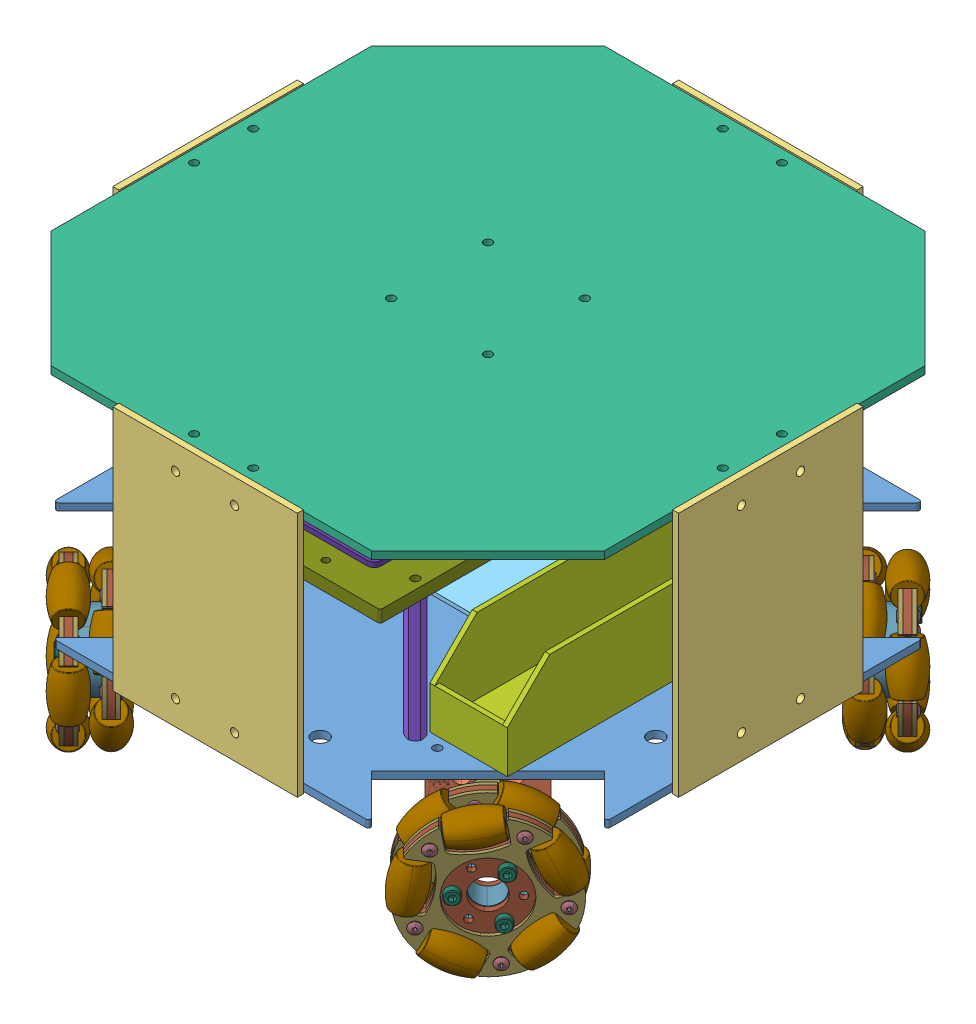
SolidWorks assembly ouijabot, configuration Default. Lengths in mm. (continued)
Components (placement in the parent): (continued)
- tx2-carrier-orbitty-1: tx2-carrier-orbitty [Default] at (43.5 74 -33.48) x (-1 0 0) z (0 -1 0) size (87.04 52.68 23.65) (continued)
  - ASG003_3D_MODEL.step-1: ASG003_3D_MODEL.step [Default] at origin size (87.04 52.68 23.65) (continued)
    - U8.step-1: U8.step [Default] at origin size (1.26 2.01 0.91) (continued)
      - 870945920.step-1: 870945920.step [Default] at (17.6522 30.9566 -2.6006) size (1.26 2.01 0.91) (continued)
        - Extruded-6.step-1: Extruded-6.step [Default] at origin size (1.26 2.01 0.91)
    - U4.step-1: U4.step [Default] at origin size (3 1.7 1.45)
      - 870946240.step-1: 870946240.step [Default] at (13.3342 34.2586 -3.0506) size (3 1.7 1.45)
        - Extruded-8.step-1: Extruded-8.step [Default] at origin size (3 1.7 1.45)
    - S1.step-1: S1.step [Default] at origin size (8.13 3.66 2.38)
      - 870942400.step-1: 870942400.step [Default] at (63.7532 2.3346 1.27) size (3.81 1.02 1.07)
        - Extruded-9.step-1: Extruded-9.step [Default] at origin size (3.81 1.02 1.07)
      - 870942560.step-1: 870942560.step [Default] at (63.7532 2.3346 1.27) size (2.54 0.76 1.09)
        - Extruded-10.step-1: Extruded-10.step [Default] at origin size (2.54 0.76 1.09)
      - 870942720.step-1: 870942720.step [Default] at (64.3247 2.3346 1.27) size (1.14 0.51 1.12)
        - Extruded-11.step-1: Extruded-11.step [Default] at origin size (1.14 0.51 1.12)
      - 870942720.step-2: 870942720.step [Default] at (63.1817 3.6046 1.27) size (1.14 0.51 1.12)
        - Extruded-11.step-1: Extruded-11.step [Default] at origin size (1.14 0.51 1.12)
      - 870942560.step-2: 870942560.step [Default] at (63.7532 3.6046 1.27) size (2.54 0.76 1.09)
        - Extruded-10.step-1: Extruded-10.step [Default] at origin size (2.54 0.76 1.09)
      - 870942400.step-2: 870942400.step [Default] at (63.7532 3.6046 1.27) size (3.81 1.02 1.07)
        - Extruded-9.step-1: Extruded-9.step [Default] at origin size (3.81 1.02 1.07)
      - c-1571983-01-b-3d.step-1: c-1571983-01-b-3d.step [Default] at (63.7533 2.9696 0.571) x (0 1 0) z (0 0 1) size (3.66 8.13 2.31)
    - R50.step-1: R50.step [Default] at origin size (0.52 1.02 0.36)
      - 870941120.step-1: 870941120.step [Default] at (22.2242 30.5266 -1.9516) size (0.52 0.16 0.35)
        - Extruded-1.step-1: Extruded-1.step [Default] at origin size (0.52 0.16 0.35)
      - 870941120.step-2: 870941120.step [Default] at (22.2242 31.3866 -1.9516) size (0.52 0.16 0.35)
        - Extruded-1.step-1: Extruded-1.step [Default] at origin size (0.52 0.16 0.35)
      - 870941280.step-1: 870941280.step [Default] at (22.2242 30.9566 -1.9506) size (0.51 1.01 0.36)
        - Extruded-2.step-1: Extruded-2.step [Default] at origin size (0.51 1.01 0.36)
    - R49.step-1: R49.step [Default] at origin size (0.52 1.02 0.36)
      - 870941120.step-1: 870941120.step [Default] at (20.9542 37.8636 -1.9516) size (0.52 0.16 0.35)
        - Extruded-1.step-1: Extruded-1.step [Default] at origin size (0.52 0.16 0.35)
      - 870941120.step-2: 870941120.step [Default] at (20.9542 37.0036 -1.9516) size (0.52 0.16 0.35)
        - Extruded-1.step-1: Extruded-1.step [Default] at origin size (0.52 0.16 0.35)
      - 870941280.step-1: 870941280.step [Default] at (20.9542 37.4336 -1.9506) size (0.51 1.01 0.36)
        - Extruded-2.step-1: Extruded-2.step [Default] at origin size (0.51 1.01 0.36)
    - R48.step-1: R48.step [Default] at origin size (0.52 1.02 0.36)
      - 870941120.step-1: 870941120.step [Default] at (21.0812 31.3866 -1.9516) size (0.52 0.16 0.35)
        - Extruded-1.step-1: Extruded-1.step [Default] at origin size (0.52 0.16 0.35)
      - 870941120.step-2: 870941120.step [Default] at (21.0812 30.5266 -1.9516) size (0.52 0.16 0.35)
        - Extruded-1.step-1: Extruded-1.step [Default] at origin size (0.52 0.16 0.35)
      - 870941280.step-1: 870941280.step [Default] at (21.0812 30.9566 -1.9506) size (0.51 1.01 0.36)
        - Extruded-2.step-1: Extruded-2.step [Default] at origin size (0.51 1.01 0.36)
    - R22.step-1: R22.step [Default] at origin size (0.52 1.02 0.36)
      - 870941120.step-1: 870941120.step [Default] at (15.3662 32.0216 -1.9516) size (0.52 0.16 0.35)
        - Extruded-1.step-1: Extruded-1.step [Default] at origin size (0.52 0.16 0.35)
      - 870941120.step-2: 870941120.step [Default] at (15.3662 31.1616 -1.9516) size (0.52 0.16 0.35)
        - Extruded-1.step-1: Extruded-1.step [Default] at origin size (0.52 0.16 0.35)
      - 870941280.step-1: 870941280.step [Default] at (15.3662 31.5916 -1.9506) size (0.51 1.01 0.36)
        - Extruded-2.step-1: Extruded-2.step [Default] at origin size (0.51 1.01 0.36)
    - R18.step-1: R18.step [Default] at origin size (0.52 1.02 0.36)
      - 870941120.step-1: 870941120.step [Default] at (78.867 21.795 -1.9516) size (0.52 0.16 0.35)
        - Extruded-1.step-1: Extruded-1.step [Default] at origin size (0.52 0.16 0.35)
      - 870941120.step-2: 870941120.step [Default] at (78.867 22.655 -1.9516) size (0.52 0.16 0.35)
        - Extruded-1.step-1: Extruded-1.step [Default] at origin size (0.52 0.16 0.35)
      - 870941280.step-1: 870941280.step [Default] at (78.867 22.225 -1.9506) size (0.51 1.01 0.36)
        - Extruded-2.step-1: Extruded-2.step [Default] at origin size (0.51 1.01 0.36)
    - L7.step-1: L7.step [Default] at origin size (1.6 0.9 0.46)
      - 870942240.step-1: 870942240.step [Default] at (75.692 25.273 -2.0506) size (1 0.9 0.45)
        - Extruded-12.step-1: Extruded-12.step [Default] at origin size (1 0.9 0.45)
      - 870942080.step-1: 870942080.step [Default] at (76.342 25.273 -2.0606) size (0.3 0.9 0.46)
        - Extruded-13.step-1: Extruded-13.step [Default] at origin size (0.3 0.9 0.46)
      - 870942080.step-2: 870942080.step [Default] at (75.042 25.273 -2.0606) size (0.3 0.9 0.46)
        - Extruded-13.step-1: Extruded-13.step [Default] at origin size (0.3 0.9 0.46)
    - C58.step-1: C58.step [Default] at origin size (0.52 1.02 0.36)
      - 870941120.step-1: 870941120.step [Default] at (19.9382 31.3866 -1.9516) size (0.52 0.16 0.35)
        - Extruded-1.step-1: Extruded-1.step [Default] at origin size (0.52 0.16 0.35)
      - 870941120.step-2: 870941120.step [Default] at (19.9382 30.5266 -1.9516) size (0.52 0.16 0.35)
        - Extruded-1.step-1: Extruded-1.step [Default] at origin size (0.52 0.16 0.35)
      - 870941280.step-1: 870941280.step [Default] at (19.9382 30.9566 -1.9506) size (0.51 1.01 0.36)
        - Extruded-2.step-1: Extruded-2.step [Default] at origin size (0.51 1.01 0.36)
    - C50.step-1: C50.step [Default] at origin size (0.52 1.02 0.36)
      - 870941120.step-1: 870941120.step [Default] at (12.4452 36.7496 -1.9516) size (0.52 0.16 0.35)
        - Extruded-1.step-1: Extruded-1.step [Default] at origin size (0.52 0.16 0.35)
      - 870941120.step-2: 870941120.step [Default] at (12.4452 37.6096 -1.9516) size (0.52 0.16 0.35)
        - Extruded-1.step-1: Extruded-1.step [Default] at origin size (0.52 0.16 0.35)
      - 870941280.step-1: 870941280.step [Default] at (12.4452 37.1796 -1.9506) size (0.51 1.01 0.36)
        - Extruded-2.step-1: Extruded-2.step [Default] at origin size (0.51 1.01 0.36)
    - C49.step-1: C49.step [Default] at origin size (0.52 1.02 0.36)
      - 870941120.step-1: 870941120.step [Default] at (14.3502 36.8076 -1.9516) size (0.52 0.16 0.35)
        - Extruded-1.step-1: Extruded-1.step [Default] at origin size (0.52 0.16 0.35)
      - 870941120.step-2: 870941120.step [Default] at (14.3502 37.6676 -1.9516) size (0.52 0.16 0.35)
        - Extruded-1.step-1: Extruded-1.step [Default] at origin size (0.52 0.16 0.35)
      - 870941280.step-1: 870941280.step [Default] at (14.3502 37.2376 -1.9506) size (0.51 1.01 0.36)
        - Extruded-2.step-1: Extruded-2.step [Default] at origin size (0.51 1.01 0.36)
    - C48.step-1: C48.step [Default] at origin size (1.02 0.52 0.36)
      - 870940480.step-1: 870940480.step [Default] at (84.533 22.733 0) size (0.16 0.52 0.35)
        - Extruded.step-1: Extruded.step [Default] at origin size (0.16 0.52 0.35)
      - 870940480.step-2: 870940480.step [Default] at (85.393 22.733 0) size (0.16 0.52 0.35)
        - Extruded.step-1: Extruded.step [Default] at origin size (0.16 0.52 0.35)
      - 870940640.step-1: 870940640.step [Default] at (84.963 22.733 0) size (1.01 0.51 0.36)
        - Extruded-0.step-1: Extruded-0.step [Default] at origin size (1.01 0.51 0.36)
    - R47.step-1: R47.step [Default] at origin size (1.02 0.52 0.36)
      - 870940480.step-1: 870940480.step [Default] at (63.9292 23.9246 0) size (0.16 0.52 0.35)
        - Extruded.step-1: Extruded.step [Default] at origin size (0.16 0.52 0.35)
      - 870940480.step-2: 870940480.step [Default] at (63.0692 23.9246 0) size (0.16 0.52 0.35)
        - Extruded.step-1: Extruded.step [Default] at origin size (0.16 0.52 0.35)
      - 870940640.step-1: 870940640.step [Default] at (63.4992 23.9246 0) size (1.01 0.51 0.36)
        - Extruded-0.step-1: Extruded-0.step [Default] at origin size (1.01 0.51 0.36)
    - R46.step-1: R46.step [Default] at origin size (0.52 1.02 0.36)
      - 870941120.step-1: 870941120.step [Default] at (8.255 20.017 0) size (0.52 0.16 0.35)
        - Extruded-1.step-1: Extruded-1.step [Default] at origin size (0.52 0.16 0.35)
      - 870941120.step-2: 870941120.step [Default] at (8.255 20.877 0) size (0.52 0.16 0.35)
        - Extruded-1.step-1: Extruded-1.step [Default] at origin size (0.52 0.16 0.35)
      - 870941280.step-1: 870941280.step [Default] at (8.255 20.447 0) size (0.51 1.01 0.36)
        - Extruded-2.step-1: Extruded-2.step [Default] at origin size (0.51 1.01 0.36)
    - L1.step-1: L1.step [Default] at origin size (1 1.25 0.29)
      - 870940800.step-1: 870940800.step [Default] at (44.881 29.538 0.005) size (1 1.25 0.29)
        - Extruded-14.step-1: Extruded-14.step [Default] at origin size (1 1.25 0.29)
    - U7.step-1: U7.step [Default] at origin size (1.6 3 1.1)
      - 870944800.step-1: 870944800.step [Default] at (65.913 27.94 0) size (1.6 3 1.1)
        - Extruded-15.step-1: Extruded-15.step [Default] at origin size (1.6 3 1.1)
    - U5.step-1: U5.step [Default] at origin size (3.1 3.1 0.95)
      - 870940320.step-1: 870940320.step [Default] at (30.2506 29.8936 0.05) size (3.1 3.1 0.95)
        - Extruded-16.step-1: Extruded-16.step [Default] at origin size (3.1 3.1 0.95)
    - U3.step-1: U3.step [Default] at origin size (3.65 3.65 0.95)
      - 870946080.step-1: 870946080.step [Default] at (8.751 30.152 -2.6006) size (3.65 3.65 0.95)
        - Extruded-17.step-1: Extruded-17.step [Default] at origin size (3.65 3.65 0.95)
    - U2.step-1: U2.step [Default] at origin size (3.65 3.65 0.95)
      - 870946080.step-1: 870946080.step [Default] at (8.751 37.539 -2.6006) size (3.65 3.65 0.95)
        - Extruded-17.step-1: Extruded-17.step [Default] at origin size (3.65 3.65 0.95)
    - U1.step-1: U1.step [Default] at origin size (4.1 4.1 0.5)
      - 870941920.step-1: 870941920.step [Default] at (55.7522 32.8146 0) size (4.1 4.1 0.5)
        - Extruded-18.step-1: Extruded-18.step [Default] at origin size (4.1 4.1 0.5)
    - SW3.step-1: SW3.step [Default] at origin size (4.6 2.8 1.9)
      - 870942880.step-1: 870942880.step [Default] at (44.9573 2.8427 0) size (4.6 2.8 1.4)
        - Extruded-19.step-1: Extruded-19.step [Default] at origin size (4.6 2.8 1.4)
      - 870943040.step-1: 870943040.step [Default] at (44.9572 2.8426 1.4) size (2.2 1.6 0.5)
        - Extruded-20.step-1: Extruded-20.step [Default] at origin size (2.2 1.6 0.5)
    - SW2.step-1: SW2.step [Default] at origin size (4.6 2.8 1.9)
      - 870942880.step-1: 870942880.step [Default] at (53.0853 2.8427 0) size (4.6 2.8 1.4)
        - Extruded-19.step-1: Extruded-19.step [Default] at origin size (4.6 2.8 1.4)
      - 870943040.step-1: 870943040.step [Default] at (53.0852 2.8426 1.4) size (2.2 1.6 0.5)
        - Extruded-20.step-1: Extruded-20.step [Default] at origin size (2.2 1.6 0.5)
    - SW1.step-1: SW1.step [Default] at origin size (4.6 2.8 1.9)
      - 870942880.step-1: 870942880.step [Default] at (36.8293 2.8427 0) size (4.6 2.8 1.4)
        - Extruded-19.step-1: Extruded-19.step [Default] at origin size (4.6 2.8 1.4)
      - 870943040.step-1: 870943040.step [Default] at (36.8292 2.8426 1.4) size (2.2 1.6 0.5)
        - Extruded-20.step-1: Extruded-20.step [Default] at origin size (2.2 1.6 0.5)
    - R45.step-1: R45.step [Default] at origin size (1.02 0.52 0.36)
      - 870940480.step-1: 870940480.step [Default] at (64.6964 25.5915 0) size (0.16 0.52 0.35)
        - Extruded.step-1: Extruded.step [Default] at origin size (0.16 0.52 0.35)
      - 870940480.step-2: 870940480.step [Default] at (65.5564 25.5915 0) size (0.16 0.52 0.35)
        - Extruded.step-1: Extruded.step [Default] at origin size (0.16 0.52 0.35)
      - 870940640.step-1: 870940640.step [Default] at (65.1264 25.5915 0) size (1.01 0.51 0.36)
        - Extruded-0.step-1: Extruded-0.step [Default] at origin size (1.01 0.51 0.36)
    - R44.step-1: R44.step [Default] at origin size (1.02 0.52 0.36)
      - 870940480.step-1: 870940480.step [Default] at (66.4744 25.5915 0) size (0.16 0.52 0.35)
        - Extruded.step-1: Extruded.step [Default] at origin size (0.16 0.52 0.35)
      - 870940480.step-2: 870940480.step [Default] at (67.3344 25.5915 0) size (0.16 0.52 0.35)
        - Extruded.step-1: Extruded.step [Default] at origin size (0.16 0.52 0.35)
      - 870940640.step-1: 870940640.step [Default] at (66.9044 25.5915 0) size (1.01 0.51 0.36)
        - Extruded-0.step-1: Extruded-0.step [Default] at origin size (1.01 0.51 0.36)
    - R39.step-1: R39.step [Default] at origin size (1.6 0.9 0.46)
      - 870942080.step-1: 870942080.step [Default] at (83.581 19.304 0) size (0.3 0.9 0.46)
        - Extruded-13.step-1: Extruded-13.step [Default] at origin size (0.3 0.9 0.46)
      - 870942080.step-2: 870942080.step [Default] at (82.281 19.304 0) size (0.3 0.9 0.46)
        - Extruded-13.step-1: Extruded-13.step [Default] at origin size (0.3 0.9 0.46)
      - 870942240.step-1: 870942240.step [Default] at (82.931 19.304 0) size (1 0.9 0.45)
        - Extruded-12.step-1: Extruded-12.step [Default] at origin size (1 0.9 0.45)
    - R38.step-1: R38.step [Default] at origin size (1.02 0.52 0.36)
      - 870940480.step-1: 870940480.step [Default] at (67.3872 19.3526 -1.9516) size (0.16 0.52 0.35)
        - Extruded.step-1: Extruded.step [Default] at origin size (0.16 0.52 0.35)
      - 870940480.step-2: 870940480.step [Default] at (68.2472 19.3526 -1.9516) size (0.16 0.52 0.35)
        - Extruded.step-1: Extruded.step [Default] at origin size (0.16 0.52 0.35)
      - 870940640.step-1: 870940640.step [Default] at (67.8172 19.3526 -1.9506) size (1.01 0.51 0.36)
        - Extruded-0.step-1: Extruded-0.step [Default] at origin size (1.01 0.51 0.36)
    - R37.step-1: R37.step [Default] at origin size (1.02 0.52 0.36)
      - 870940480.step-1: 870940480.step [Default] at (61.3892 19.3526 -1.9516) size (0.16 0.52 0.35)
        - Extruded.step-1: Extruded.step [Default] at origin size (0.16 0.52 0.35)
      - 870940480.step-2: 870940480.step [Default] at (60.5292 19.3526 -1.9516) size (0.16 0.52 0.35)
        - Extruded.step-1: Extruded.step [Default] at origin size (0.16 0.52 0.35)
      - 870940640.step-1: 870940640.step [Default] at (60.9592 19.3526 -1.9506) size (1.01 0.51 0.36)
        - Extruded-0.step-1: Extruded-0.step [Default] at origin size (1.01 0.51 0.36)
    - R36.step-1: R36.step [Default] at origin size (1.02 0.52 0.36)
      - 870940480.step-1: 870940480.step [Default] at (64.9742 23.9246 0) size (0.16 0.52 0.35)
        - Extruded.step-1: Extruded.step [Default] at origin size (0.16 0.52 0.35)
      - 870940480.step-2: 870940480.step [Default] at (65.8342 23.9246 0) size (0.16 0.52 0.35)
        - Extruded.step-1: Extruded.step [Default] at origin size (0.16 0.52 0.35)
      - 870940640.step-1: 870940640.step [Default] at (65.4042 23.9246 0) size (1.01 0.51 0.36)
        - Extruded-0.step-1: Extruded-0.step [Default] at origin size (1.01 0.51 0.36)
    - R35.step-1: R35.step [Default] at origin size (0.52 1.02 0.36)
      - 870941120.step-1: 870941120.step [Default] at (32.0286 29.6596 -1.9516) size (0.52 0.16 0.35)
        - Extruded-1.step-1: Extruded-1.step [Default] at origin size (0.52 0.16 0.35)
      - 870941120.step-2: 870941120.step [Default] at (32.0286 30.5196 -1.9516) size (0.52 0.16 0.35)
        - Extruded-1.step-1: Extruded-1.step [Default] at origin size (0.52 0.16 0.35)
      - 870941280.step-1: 870941280.step [Default] at (32.0286 30.0896 -1.9506) size (0.51 1.01 0.36)
        - Extruded-2.step-1: Extruded-2.step [Default] at origin size (0.51 1.01 0.36)
    - R34.step-1: R34.step [Default] at origin size (1.02 0.52 0.36)
      - 870940480.step-1: 870940480.step [Default] at (32.865 28.6744 -1.9516) size (0.16 0.52 0.35)
        - Extruded.step-1: Extruded.step [Default] at origin size (0.16 0.52 0.35)
      - 870940480.step-2: 870940480.step [Default] at (32.005 28.6744 -1.9516) size (0.16 0.52 0.35)
        - Extruded.step-1: Extruded.step [Default] at origin size (0.16 0.52 0.35)
      - 870940640.step-1: 870940640.step [Default] at (32.435 28.6744 -1.9506) size (1.01 0.51 0.36)
        - Extruded-0.step-1: Extruded-0.step [Default] at origin size (1.01 0.51 0.36)
    - R33.step-1: R33.step [Default] at origin size (1.02 0.52 0.36)
      - 870940480.step-1: 870940480.step [Default] at (69.695 43.127 0) size (0.16 0.52 0.35)
        - Extruded.step-1: Extruded.step [Default] at origin size (0.16 0.52 0.35)
      - 870940480.step-2: 870940480.step [Default] at (68.835 43.127 0) size (0.16 0.52 0.35)
        - Extruded.step-1: Extruded.step [Default] at origin size (0.16 0.52 0.35)
      - 870940640.step-1: 870940640.step [Default] at (69.265 43.127 0) size (1.01 0.51 0.36)
        - Extruded-0.step-1: Extruded-0.step [Default] at origin size (1.01 0.51 0.36)
    - R32.step-1: R32.step [Default] at origin size (1.02 0.52 0.36)
      - 870940480.step-1: 870940480.step [Default] at (30.6806 31.2906 -1.9516) size (0.16 0.52 0.35)
        - Extruded.step-1: Extruded.step [Default] at origin size (0.16 0.52 0.35)
      - 870940480.step-2: 870940480.step [Default] at (29.8206 31.2906 -1.9516) size (0.16 0.52 0.35)
        - Extruded.step-1: Extruded.step [Default] at origin size (0.16 0.52 0.35)
      - 870940640.step-1: 870940640.step [Default] at (30.2506 31.2906 -1.9506) size (1.01 0.51 0.36)
        - Extruded-0.step-1: Extruded-0.step [Default] at origin size (1.01 0.51 0.36)
    - R31.step-1: R31.step [Default] at origin size (0.52 1.02 0.36)
      - 870941120.step-1: 870941120.step [Default] at (28.4726 29.7176 -1.9516) size (0.52 0.16 0.35)
        - Extruded-1.step-1: Extruded-1.step [Default] at origin size (0.52 0.16 0.35)
      - 870941120.step-2: 870941120.step [Default] at (28.4726 30.5776 -1.9516) size (0.52 0.16 0.35)
        - Extruded-1.step-1: Extruded-1.step [Default] at origin size (0.52 0.16 0.35)
      - 870941280.step-1: 870941280.step [Default] at (28.4726 30.1476 -1.9506) size (0.51 1.01 0.36)
        - Extruded-2.step-1: Extruded-2.step [Default] at origin size (0.51 1.01 0.36)
    - R30.step-1: R30.step [Default] at origin size (1.02 0.52 0.36)
      - 870940480.step-1: 870940480.step [Default] at (27.6362 28.6998 -1.9516) size (0.16 0.52 0.35)
        - Extruded.step-1: Extruded.step [Default] at origin size (0.16 0.52 0.35)
      - 870940480.step-2: 870940480.step [Default] at (28.4962 28.6998 -1.9516) size (0.16 0.52 0.35)
        - Extruded.step-1: Extruded.step [Default] at origin size (0.16 0.52 0.35)
      - 870940640.step-1: 870940640.step [Default] at (28.0662 28.6998 -1.9506) size (1.01 0.51 0.36)
        - Extruded-0.step-1: Extruded-0.step [Default] at origin size (1.01 0.51 0.36)
    - R29.step-1: R29.step [Default] at origin size (0.52 1.02 0.36)
      - 870941120.step-1: 870941120.step [Default] at (68.884 46.224 0) size (0.52 0.16 0.35)
        - Extruded-1.step-1: Extruded-1.step [Default] at origin size (0.52 0.16 0.35)
      - 870941120.step-2: 870941120.step [Default] at (68.884 45.364 0) size (0.52 0.16 0.35)
        - Extruded-1.step-1: Extruded-1.step [Default] at origin size (0.52 0.16 0.35)
      - 870941280.step-1: 870941280.step [Default] at (68.884 45.794 0) size (0.51 1.01 0.36)
        - Extruded-2.step-1: Extruded-2.step [Default] at origin size (0.51 1.01 0.36)
    - R28.step-1: R28.step [Default] at origin size (0.52 1.02 0.36)
      - 870941120.step-1: 870941120.step [Default] at (51.054 8.333 0) size (0.52 0.16 0.35)
        - Extruded-1.step-1: Extruded-1.step [Default] at origin size (0.52 0.16 0.35)
      - 870941120.step-2: 870941120.step [Default] at (51.054 9.193 0) size (0.52 0.16 0.35)
        - Extruded-1.step-1: Extruded-1.step [Default] at origin size (0.52 0.16 0.35)
      - 870941280.step-1: 870941280.step [Default] at (51.054 8.763 0) size (0.51 1.01 0.36)
        - Extruded-2.step-1: Extruded-2.step [Default] at origin size (0.51 1.01 0.36)
    - R27.step-1: R27.step [Default] at origin size (0.52 1.02 0.36)
      - 870941120.step-1: 870941120.step [Default] at (50.038 9.193 0) size (0.52 0.16 0.35)
        - Extruded-1.step-1: Extruded-1.step [Default] at origin size (0.52 0.16 0.35)
      - 870941120.step-2: 870941120.step [Default] at (50.038 8.333 0) size (0.52 0.16 0.35)
        - Extruded-1.step-1: Extruded-1.step [Default] at origin size (0.52 0.16 0.35)
      - 870941280.step-1: 870941280.step [Default] at (50.038 8.763 0) size (0.51 1.01 0.36)
        - Extruded-2.step-1: Extruded-2.step [Default] at origin size (0.51 1.01 0.36)
    - R26.step-1: R26.step [Default] at origin size (0.52 1.02 0.36)
      - 870941120.step-1: 870941120.step [Default] at (73.66 34.466 -1.9516) size (0.52 0.16 0.35)
        - Extruded-1.step-1: Extruded-1.step [Default] at origin size (0.52 0.16 0.35)
      - 870941120.step-2: 870941120.step [Default] at (73.66 33.606 -1.9516) size (0.52 0.16 0.35)
        - Extruded-1.step-1: Extruded-1.step [Default] at origin size (0.52 0.16 0.35)
      - 870941280.step-1: 870941280.step [Default] at (73.66 34.036 -1.9506) size (0.51 1.01 0.36)
        - Extruded-2.step-1: Extruded-2.step [Default] at origin size (0.51 1.01 0.36)
    - R25.step-1: R25.step [Default] at origin size (1.02 0.52 0.36)
      - 870940480.step-1: 870940480.step [Default] at (78.183 29.337 -1.9516) size (0.16 0.52 0.35)
        - Extruded.step-1: Extruded.step [Default] at origin size (0.16 0.52 0.35)
      - 870940480.step-2: 870940480.step [Default] at (79.043 29.337 -1.9516) size (0.16 0.52 0.35)
        - Extruded.step-1: Extruded.step [Default] at origin size (0.16 0.52 0.35)
      - 870940640.step-1: 870940640.step [Default] at (78.613 29.337 -1.9506) size (1.01 0.51 0.36)
        - Extruded-0.step-1: Extruded-0.step [Default] at origin size (1.01 0.51 0.36)
    - R24.step-1: R24.step [Default] at origin size (0.52 1.02 0.36)
      - 870941120.step-1: 870941120.step [Default] at (20.878 18.694 -1.9516) size (0.52 0.16 0.35)
        - Extruded-1.step-1: Extruded-1.step [Default] at origin size (0.52 0.16 0.35)
      - 870941120.step-2: 870941120.step [Default] at (20.878 19.554 -1.9516) size (0.52 0.16 0.35)
        - Extruded-1.step-1: Extruded-1.step [Default] at origin size (0.52 0.16 0.35)
      - 870941280.step-1: 870941280.step [Default] at (20.878 19.124 -1.9506) size (0.51 1.01 0.36)
        - Extruded-2.step-1: Extruded-2.step [Default] at origin size (0.51 1.01 0.36)
    - R23.step-1: R23.step [Default] at origin size (0.52 1.02 0.36)
      - 870941120.step-1: 870941120.step [Default] at (10.464 18.694 -1.9516) size (0.52 0.16 0.35)
        - Extruded-1.step-1: Extruded-1.step [Default] at origin size (0.52 0.16 0.35)
      - 870941120.step-2: 870941120.step [Default] at (10.464 19.554 -1.9516) size (0.52 0.16 0.35)
        - Extruded-1.step-1: Extruded-1.step [Default] at origin size (0.52 0.16 0.35)
      - 870941280.step-1: 870941280.step [Default] at (10.464 19.124 -1.9506) size (0.51 1.01 0.36)
        - Extruded-2.step-1: Extruded-2.step [Default] at origin size (0.51 1.01 0.36)
    - R20.step-1: R20.step [Default] at origin size (1.02 0.52 0.36)
      - 870940480.step-1: 870940480.step [Default] at (7.854 26.67 -1.9516) size (0.16 0.52 0.35)
        - Extruded.step-1: Extruded.step [Default] at origin size (0.16 0.52 0.35)
      - 870940480.step-2: 870940480.step [Default] at (6.994 26.67 -1.9516) size (0.16 0.52 0.35)
        - Extruded.step-1: Extruded.step [Default] at origin size (0.16 0.52 0.35)
      - 870940640.step-1: 870940640.step [Default] at (7.424 26.67 -1.9506) size (1.01 0.51 0.36)
        - Extruded-0.step-1: Extruded-0.step [Default] at origin size (1.01 0.51 0.36)
    - R21.step-1: R21.step [Default] at origin size (1.02 0.52 0.36)
      - 870940480.step-1: 870940480.step [Default] at (18.8442 37.0526 -1.9516) size (0.16 0.52 0.35)
        - Extruded.step-1: Extruded.step [Default] at origin size (0.16 0.52 0.35)
      - 870940480.step-2: 870940480.step [Default] at (17.9842 37.0526 -1.9516) size (0.16 0.52 0.35)
        - Extruded.step-1: Extruded.step [Default] at origin size (0.16 0.52 0.35)
      - 870940640.step-1: 870940640.step [Default] at (18.4142 37.0526 -1.9506) size (1.01 0.51 0.36)
        - Extruded-0.step-1: Extruded-0.step [Default] at origin size (1.01 0.51 0.36)
    - R19.step-1: R19.step [Default] at origin size (0.52 1.02 0.36)
      - 870941120.step-1: 870941120.step [Default] at (55.372 8.431 0) size (0.52 0.16 0.35)
        - Extruded-1.step-1: Extruded-1.step [Default] at origin size (0.52 0.16 0.35)
      - 870941120.step-2: 870941120.step [Default] at (55.372 7.571 0) size (0.52 0.16 0.35)
        - Extruded-1.step-1: Extruded-1.step [Default] at origin size (0.52 0.16 0.35)
      - 870941280.step-1: 870941280.step [Default] at (55.372 8.001 0) size (0.51 1.01 0.36)
        - Extruded-2.step-1: Extruded-2.step [Default] at origin size (0.51 1.01 0.36)
    - R15.step-1: R15.step [Default] at origin size (1.02 0.52 0.36)
      - 870940480.step-1: 870940480.step [Default] at (7.923 34.671 -1.9516) size (0.16 0.52 0.35)
        - Extruded.step-1: Extruded.step [Default] at origin size (0.16 0.52 0.35)
      - 870940480.step-2: 870940480.step [Default] at (7.063 34.671 -1.9516) size (0.16 0.52 0.35)
        - Extruded.step-1: Extruded.step [Default] at origin size (0.16 0.52 0.35)
      - 870940640.step-1: 870940640.step [Default] at (7.493 34.671 -1.9506) size (1.01 0.51 0.36)
        - Extruded-0.step-1: Extruded-0.step [Default] at origin size (1.01 0.51 0.36)
    - R17.step-1: R17.step [Default] at origin size (0.52 1.02 0.36)
      - 870941120.step-1: 870941120.step [Default] at (54.356 7.571 0) size (0.52 0.16 0.35)
        - Extruded-1.step-1: Extruded-1.step [Default] at origin size (0.52 0.16 0.35)
      - 870941120.step-2: 870941120.step [Default] at (54.356 8.431 0) size (0.52 0.16 0.35)
        - Extruded-1.step-1: Extruded-1.step [Default] at origin size (0.52 0.16 0.35)
      - 870941280.step-1: 870941280.step [Default] at (54.356 8.001 0) size (0.51 1.01 0.36)
        - Extruded-2.step-1: Extruded-2.step [Default] at origin size (0.51 1.01 0.36)
    - R16.step-1: R16.step [Default] at origin size (0.52 1.02 0.36)
      - 870941120.step-1: 870941120.step [Default] at (82.931 22.245 0) size (0.52 0.16 0.35)
        - Extruded-1.step-1: Extruded-1.step [Default] at origin size (0.52 0.16 0.35)
      - 870941120.step-2: 870941120.step [Default] at (82.931 23.105 0) size (0.52 0.16 0.35)
        - Extruded-1.step-1: Extruded-1.step [Default] at origin size (0.52 0.16 0.35)
      - 870941280.step-1: 870941280.step [Default] at (82.931 22.675 0) size (0.51 1.01 0.36)
        - Extruded-2.step-1: Extruded-2.step [Default] at origin size (0.51 1.01 0.36)
    - R11.step-1: R11.step [Default] at origin size (1.02 0.52 0.36)
      - 870940480.step-1: 870940480.step [Default] at (52.4738 26.4392 0) size (0.16 0.52 0.35)
        - Extruded.step-1: Extruded.step [Default] at origin size (0.16 0.52 0.35)
      - 870940480.step-2: 870940480.step [Default] at (51.6138 26.4392 0) size (0.16 0.52 0.35)
        - Extruded.step-1: Extruded.step [Default] at origin size (0.16 0.52 0.35)
      - 870940640.step-1: 870940640.step [Default] at (52.0438 26.4392 0) size (1.01 0.51 0.36)
        - Extruded-0.step-1: Extruded-0.step [Default] at origin size (1.01 0.51 0.36)
    - R10.step-1: R10.step [Default] at origin size (1.02 0.52 0.36)
      - 870940480.step-1: 870940480.step [Default] at (49.8358 26.4392 0) size (0.16 0.52 0.35)
        - Extruded.step-1: Extruded.step [Default] at origin size (0.16 0.52 0.35)
      - 870940480.step-2: 870940480.step [Default] at (50.6958 26.4392 0) size (0.16 0.52 0.35)
        - Extruded.step-1: Extruded.step [Default] at origin size (0.16 0.52 0.35)
      - 870940640.step-1: 870940640.step [Default] at (50.2658 26.4392 0) size (1.01 0.51 0.36)
        - Extruded-0.step-1: Extruded-0.step [Default] at origin size (1.01 0.51 0.36)
    - R9.step-1: R9.step [Default] at origin size (1.02 0.52 0.36)
      - 870940480.step-1: 870940480.step [Default] at (55.2678 27.4552 0) size (0.16 0.52 0.35)
        - Extruded.step-1: Extruded.step [Default] at origin size (0.16 0.52 0.35)
      - 870940480.step-2: 870940480.step [Default] at (54.4078 27.4552 0) size (0.16 0.52 0.35)
        - Extruded.step-1: Extruded.step [Default] at origin size (0.16 0.52 0.35)
      - 870940640.step-1: 870940640.step [Default] at (54.8378 27.4552 0) size (1.01 0.51 0.36)
        - Extruded-0.step-1: Extruded-0.step [Default] at origin size (1.01 0.51 0.36)
    - R8.step-1: R8.step [Default] at origin size (1.02 0.52 0.36)
      - 870940480.step-1: 870940480.step [Default] at (52.6298 27.4552 0) size (0.16 0.52 0.35)
        - Extruded.step-1: Extruded.step [Default] at origin size (0.16 0.52 0.35)
      - 870940480.step-2: 870940480.step [Default] at (53.4898 27.4552 0) size (0.16 0.52 0.35)
        - Extruded.step-1: Extruded.step [Default] at origin size (0.16 0.52 0.35)
      - 870940640.step-1: 870940640.step [Default] at (53.0598 27.4552 0) size (1.01 0.51 0.36)
        - Extruded-0.step-1: Extruded-0.step [Default] at origin size (1.01 0.51 0.36)
    - R7.step-1: R7.step [Default] at origin size (1.02 0.52 0.36)
      - 870940480.step-1: 870940480.step [Default] at (58.0618 26.4392 0) size (0.16 0.52 0.35)
        - Extruded.step-1: Extruded.step [Default] at origin size (0.16 0.52 0.35)
      - 870940480.step-2: 870940480.step [Default] at (57.2018 26.4392 0) size (0.16 0.52 0.35)
        - Extruded.step-1: Extruded.step [Default] at origin size (0.16 0.52 0.35)
      - 870940640.step-1: 870940640.step [Default] at (57.6318 26.4392 0) size (1.01 0.51 0.36)
        - Extruded-0.step-1: Extruded-0.step [Default] at origin size (1.01 0.51 0.36)
    - R6.step-1: R6.step [Default] at origin size (1.02 0.52 0.36)
      - 870940480.step-1: 870940480.step [Default] at (55.4238 26.4392 0) size (0.16 0.52 0.35)
        - Extruded.step-1: Extruded.step [Default] at origin size (0.16 0.52 0.35)
      - 870940480.step-2: 870940480.step [Default] at (56.2838 26.4392 0) size (0.16 0.52 0.35)
        - Extruded.step-1: Extruded.step [Default] at origin size (0.16 0.52 0.35)
      - 870940640.step-1: 870940640.step [Default] at (55.8538 26.4392 0) size (1.01 0.51 0.36)
        - Extruded-0.step-1: Extruded-0.step [Default] at origin size (1.01 0.51 0.36)
    - R5.step-1: R5.step [Default] at origin size (1.02 0.52 0.36)
      - 870940480.step-1: 870940480.step [Default] at (60.8558 27.4552 0) size (0.16 0.52 0.35)
        - Extruded.step-1: Extruded.step [Default] at origin size (0.16 0.52 0.35)
      - 870940480.step-2: 870940480.step [Default] at (59.9958 27.4552 0) size (0.16 0.52 0.35)
        - Extruded.step-1: Extruded.step [Default] at origin size (0.16 0.52 0.35)
      - 870940640.step-1: 870940640.step [Default] at (60.4258 27.4552 0) size (1.01 0.51 0.36)
        - Extruded-0.step-1: Extruded-0.step [Default] at origin size (1.01 0.51 0.36)
    - R4.step-1: R4.step [Default] at origin size (1.02 0.52 0.36)
      - 870940480.step-1: 870940480.step [Default] at (58.2178 27.4552 0) size (0.16 0.52 0.35)
        - Extruded.step-1: Extruded.step [Default] at origin size (0.16 0.52 0.35)
      - 870940480.step-2: 870940480.step [Default] at (59.0778 27.4552 0) size (0.16 0.52 0.35)
        - Extruded.step-1: Extruded.step [Default] at origin size (0.16 0.52 0.35)
      - 870940640.step-1: 870940640.step [Default] at (58.6478 27.4552 0) size (1.01 0.51 0.36)
        - Extruded-0.step-1: Extruded-0.step [Default] at origin size (1.01 0.51 0.36)
    - R3.step-1: R3.step [Default] at origin size (1.02 0.52 0.36)
      - 870940480.step-1: 870940480.step [Default] at (56.3644 29.2354 -1.9516) size (0.16 0.52 0.35)
        - Extruded.step-1: Extruded.step [Default] at origin size (0.16 0.52 0.35)
      - 870940480.step-2: 870940480.step [Default] at (57.2244 29.2354 -1.9516) size (0.16 0.52 0.35)
        - Extruded.step-1: Extruded.step [Default] at origin size (0.16 0.52 0.35)
      - 870940640.step-1: 870940640.step [Default] at (56.7944 29.2354 -1.9506) size (1.01 0.51 0.36)
        - Extruded-0.step-1: Extruded-0.step [Default] at origin size (1.01 0.51 0.36)
    - R2.step-1: R2.step [Default] at origin size (0.52 1.02 0.36)
      - 870941120.step-1: 870941120.step [Default] at (59.055 36.654 0) size (0.52 0.16 0.35)
        - Extruded-1.step-1: Extruded-1.step [Default] at origin size (0.52 0.16 0.35)
      - 870941120.step-2: 870941120.step [Default] at (59.055 37.514 0) size (0.52 0.16 0.35)
        - Extruded-1.step-1: Extruded-1.step [Default] at origin size (0.52 0.16 0.35)
      - 870941280.step-1: 870941280.step [Default] at (59.055 37.084 0) size (0.51 1.01 0.36)
        - Extruded-2.step-1: Extruded-2.step [Default] at origin size (0.51 1.01 0.36)
    - R1.step-1: R1.step [Default] at origin size (1.02 0.52 0.36)
      - 870940480.step-1: 870940480.step [Default] at (52.5246 33.0432 0) size (0.16 0.52 0.35)
        - Extruded.step-1: Extruded.step [Default] at origin size (0.16 0.52 0.35)
      - 870940480.step-2: 870940480.step [Default] at (51.6646 33.0432 0) size (0.16 0.52 0.35)
        - Extruded.step-1: Extruded.step [Default] at origin size (0.16 0.52 0.35)
      - 870940640.step-1: 870940640.step [Default] at (52.0946 33.0432 0) size (1.01 0.51 0.36)
        - Extruded-0.step-1: Extruded-0.step [Default] at origin size (1.01 0.51 0.36)
    - Q6.step-1: Q6.step [Default] at origin size (6.7 7.2 3)
      - 870943520.step-1: 870943520.step [Default] at (74.8022 10.3156 0) size (5.4 1.25 1)
        - Extruded-21.step-1: Extruded-21.step [Default] at origin size (5.4 1.25 1)
      - 870943680.step-1: 870943680.step [Default] at (74.8522 13.9406 0) size (6.7 5.9 3)
        - Extruded-22.step-1: Extruded-22.step [Default] at origin size (6.7 5.9 3)
    - Q4.step-1: Q4.step [Default] at origin size (2.42 2.9 1)
      - SW3dPS-SOT-23.step-1: SW3dPS-SOT-23.step [Default] at (58.9281 7.1121 0.498) x (-1 0 0) z (0 1 0) size (2.42 1 2.9)
    - Q3.step-1: Q3.step [Default] at origin size (2.9 2.42 1)
      - SW3dPS-SOT-23.step-1: SW3dPS-SOT-23.step [Default] at (10.5411 3.81 0.498) x (0 1 0) z (1 0 0) size (2.42 1 2.9)
    - Q2.step-1: Q2.step [Default] at origin size (2.9 2.42 1)
      - SW3dPS-SOT-23.step-1: SW3dPS-SOT-23.step [Default] at (53.7201 29.2332 -2.0986) x (0 1 0) z (-1 0 0) size (2.42 1 2.9)
    - Q1.step-1: Q1.step [Default] at origin size (2.9 2.42 1)
      - SW3dPS-SOT-23.step-1: SW3dPS-SOT-23.step [Default] at (48.3615 24.8667 0.498) x (0 -1 0) z (-1 0 0) size (2.42 1 2.9)
    - P8.step-1: P8.step [Default] at origin size (8 5.6 3.08)
      - c-1981568-1-c-3d.step-1: c-1981568-1-c-3d.step [Default] at (74.172 50.762 1.2552) x (-1 0 0) z (0 1 0) size (8 3.08 5.6)
    - P7.step-1: P7.step [Default] at origin size (16.11 16.48 11.74)
      - c-1932258-1-a-3d.step-1: c-1932258-1-a-3d.step [Default] at (38.1659 51.3109 4.1452) x (-1 0 0) z (0 1 0) size (16.11 11.74 16.48)
    - P6.step-1: P6.step [Default] at origin size (15.5 13.8 1.8)
      - 5025700893.step-1: 5025700893.step [Default] at (17.2345 76.9985 0.9152) x (0 -1 0) z (0 0 1) size (13.8 15.5 1.8)
        - Open CASCADE STEP translator 6.8 1.83.1.1.step-1: Open CASCADE STEP translator 6.8 1.83.1.1.step [Default] at origin size (13.8 15.5 1.8)
        - Open CASCADE STEP translator 6.8 1.83.1.2.step-1: Open CASCADE STEP translator 6.8 1.83.1.2.step [Default] at origin
    - P5.step-1: P5.step [Default] at origin size (19.89 33.03 18.91)
      - User_Library-WE-RJ45_LAN_HPLE_RJ45_LAN_Transformer_799111614_W_rthElektronik.step-1: User_Library-WE-RJ45_LAN_HPLE_RJ45_LAN_Transformer_799111614_W_rthElektronik.step [Default] at (17.7218 36.1528 0.0152) x (-1 0 0) z (0 1 0) size (19.89 18.91 33.03)
    - P4.step-1: P4.step [Default] at origin size (5.08 25.4 10.92)
      - Samtec-TSW-110-07-L-D.step-1: Samtec-TSW-110-07-L-D.step [Default] at (3.429 19.05 0) x (0 -1 0) z (-1 0 0) size (25.4 10.92 5.08)
    - P3.step-1: P3.step [Default] at origin size (5.12 9.75 3.4)
      - S-50271-004xx-xxx_RGB5527646.step-1: S-50271-004xx-xxx_RGB5527646.step [Default] at (82.288 23.358 -3.3006) x (0 1 0) z (0 0 -1) size (9.75 5.12 3.4)
        - Open CASCADE STEP translator 6.8 1.86.1.1.step-1: Open CASCADE STEP translator 6.8 1.86.1.1.step [Default] at origin size (9.75 5.12 3.4)
        - Open CASCADE STEP translator 6.8 1.86.1.2.step-1: Open CASCADE STEP translator 6.8 1.86.1.2.step [Default] at origin
    - P2.step-1: P2.step [Default] at origin size (15 12 8.28)
      - c-1747981-1-f2-3d.step-1: c-1747981-1-f2-3d.step [Default] at (57.51 51.35 3.2202) x (-1 0 0) z (0 1 0) size (15 8.28 12)
    - L6.step-1: L6.step [Default] at origin size (0.9 1.6 0.46)
      - 870944160.step-1: 870944160.step [Default] at (67.36 45.032 0) size (0.9 1 0.45)
        - Extruded-23.step-1: Extruded-23.step [Default] at origin size (0.9 1 0.45)
      - 870944320.step-1: 870944320.step [Default] at (67.36 45.682 0) size (0.9 0.3 0.46)
        - Extruded-24.step-1: Extruded-24.step [Default] at origin size (0.9 0.3 0.46)
      - 870944320.step-2: 870944320.step [Default] at (67.36 44.382 0) size (0.9 0.3 0.46)
        - Extruded-24.step-1: Extruded-24.step [Default] at origin size (0.9 0.3 0.46)
    - L5.step-1: L5.step [Default] at origin size (0.9 1.6 0.46)
      - 870944160.step-1: 870944160.step [Default] at (41.071 40.587 -2.0506) size (0.9 1 0.45)
        - Extruded-23.step-1: Extruded-23.step [Default] at origin size (0.9 1 0.45)
      - 870944320.step-1: 870944320.step [Default] at (41.071 39.937 -2.0606) size (0.9 0.3 0.46)
        - Extruded-24.step-1: Extruded-24.step [Default] at origin size (0.9 0.3 0.46)
      - 870944320.step-2: 870944320.step [Default] at (41.071 41.237 -2.0606) size (0.9 0.3 0.46)
        - Extruded-24.step-1: Extruded-24.step [Default] at origin size (0.9 0.3 0.46)
    - L4.step-1: L4.step [Default] at origin size (1.25 1 0.29)
      - 870944000.step-1: 870944000.step [Default] at (71.7542 41.5776 0.005) size (1.25 1 0.29)
        - Extruded-25.step-1: Extruded-25.step [Default] at origin size (1.25 1 0.29)
    - L3.step-1: L3.step [Default] at origin size (1 1.25 0.29)
      - 870940800.step-1: 870940800.step [Default] at (41.166 29.531 0.005) size (1 1.25 0.29)
        - Extruded-14.step-1: Extruded-14.step [Default] at origin size (1 1.25 0.29)
    - L2.step-1: L2.step [Default] at origin size (1 1.25 0.29)
      - 870940800.step-1: 870940800.step [Default] at (35.166 29.531 0.005) size (1 1.25 0.29)
        - Extruded-14.step-1: Extruded-14.step [Default] at origin size (1 1.25 0.29)
    - F1.step-1: F1.step [Default] at origin size (4.6 3.2 0.7)
      - 870945440.step-1: 870945440.step [Default] at (78.613 32.258 -2.3006) size (4 3.2 0.7)
        - Extruded-26.step-1: Extruded-26.step [Default] at origin size (4 3.2 0.7)
      - 870945600.step-1: 870945600.step [Default] at (76.463 32.258 -2.3006) size (0.3 3.2 0.7)
        - Extruded-27.step-1: Extruded-27.step [Default] at origin size (0.3 3.2 0.7)
      - 870945600.step-2: 870945600.step [Default] at (80.763 32.258 -2.3006) size (0.3 3.2 0.7)
        - Extruded-27.step-1: Extruded-27.step [Default] at origin size (0.3 3.2 0.7)
    - D11.step-1: D11.step [Default] at origin size (1.02 0.52 0.36)
      - 870944640.step-1: 870944640.step [Default] at (15.6202 1.0646 0) size (1.01 0.51 0.36)
        - Extruded-28.step-1: Extruded-28.step [Default] at origin size (1.01 0.51 0.36)
      - 870940480.step-1: 870940480.step [Default] at (15.1902 1.0646 0) size (0.16 0.52 0.35)
        - Extruded.step-1: Extruded.step [Default] at origin size (0.16 0.52 0.35)
      - 870940480.step-2: 870940480.step [Default] at (16.0502 1.0646 0) size (0.16 0.52 0.35)
        - Extruded.step-1: Extruded.step [Default] at origin size (0.16 0.52 0.35)
    - D10.step-1: D10.step [Default] at origin size (2.6 5.21 2.46)
      - User_Library-DO-214AC_SMA.step-1: User_Library-DO-214AC_SMA.step [Default] at (80.5181 13.8429 -3.0159) x (1 0 0) z (0 0 -1) size (2.6 5.21 2.46)
    - D9.step-1: D9.step [Default] at origin size (1.5 1.95 1.15)
      - 870943840.step-1: 870943840.step [Default] at (80.0092 19.4796 0) size (1.5 1.95 1.15)
        - Extruded-29.step-1: Extruded-29.step [Default] at origin size (1.5 1.95 1.15)
    - D8.step-1: D8.step [Default] at origin size (1.1 0.7 0.55)
      - 870944480.step-1: 870944480.step [Default] at (76.885 41.857 0) size (1.1 0.7 0.55)
